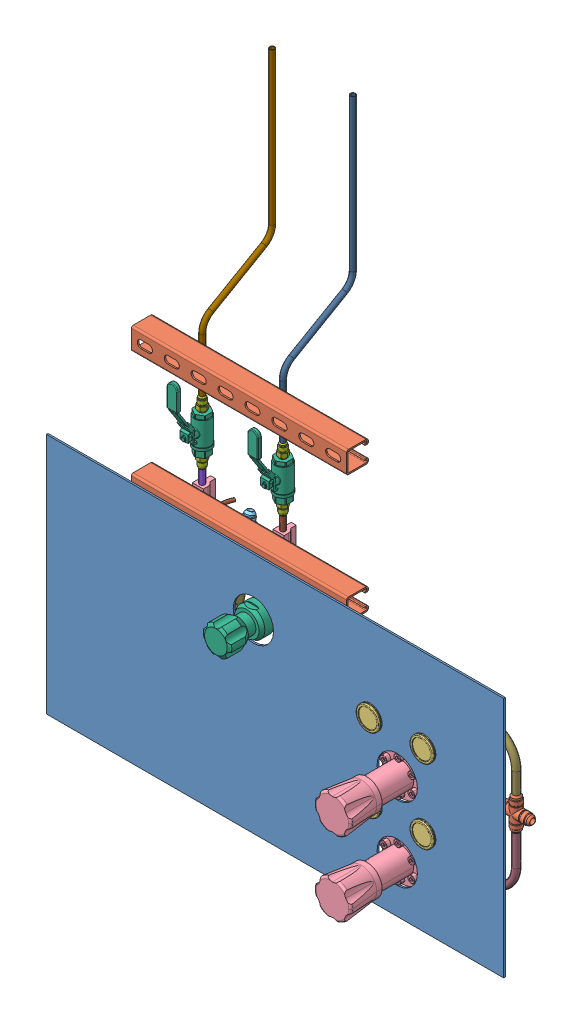
SolidWorks assembly N2_panel, configuration Default. Lengths in mm.
Overall size (886.81 1079.1 374.6).
81 component instances, 31 part files, 49 mates.
Components (placement in the parent):
- N2_panel-1: N2_panel [Default] at origin size (863.6 457.2 3.17)
- SS-2650-08-08-08-08-1: SS-2650-08-08-08-08 [5482K249] at (400.8501 0 -51.435) size (81.9 81.9 19.05)
- 9780T219_VIBRATION-RESISTANT PRESSURE GAUGE-3: 9780T219_VIBRATION-RESISTANT PRESSURE GAUGE [9780T219] at (179.9381 -67.2228 8.636) x (-1 0 0) z (0 0 1) size (44.45 61.91 48.07)
- 9780T219_VIBRATION-RESISTANT PRESSURE GAUGE-4: 9780T219_VIBRATION-RESISTANT PRESSURE GAUGE [9780T219] at (281.5381 -67.2228 8.636) x (-1 0 0) z (0 0 1) size (44.45 61.91 48.07)
- PRV-1 & PRV-2 Assembly-1: PRV-1 & PRV-2 Assembly [Default] at (230.7381 -139.7 -104.521) size (144.32 78.02 230.14)
  - PRV-1&2_RSHN4-02-6-VVK-Swagelok-1: PRV-1&2_RSHN4-02-6-VVK-Swagelok [Default] at origin size (72 78.02 230.14)
  - 50715K166_TYPE 316 SS 37 DEGREE FLARED TUBE FITTING-1: 50715K166_TYPE 316 SS 37 DEGREE FLARED TUBE FITTING [50715K802] at (39.556 0 53.086) x (1 0 0) z (0 0.0006 1) size (55.21 25.66 22.23)
  - 50715K166_TYPE 316 SS 37 DEGREE FLARED TUBE FITTING-2: 50715K166_TYPE 316 SS 37 DEGREE FLARED TUBE FITTING [50715K802] at (-39.556 0 53.086) x (-1 0 0) z (0 -0.0006 -1) size (55.21 25.66 22.23)
- PRV-3 Assembly-1: PRV-3 Assembly [Default] at (-40.8559 120.65 -138.049) x (-1 0 0) z (0 0 1) size (149.78 55.88 212.09)
  - KCY1JPA412A20000_PRT_29-1: KCY1JPA412A20000_PRT_29 [Default] at origin size (56.39 55.88 212.09)
  - 51205K317_EXTREME-PRESSURE 316 SS THREADED PIPE FITTING-1: 51205K317_EXTREME-PRESSURE 316 SS THREADED PIPE FITTING [51205K317] at (-34.807 0 86.614) x (-1 0 0) z (0 0.601506 -0.798868) size (42.93 32.74 28.57)
  - 50715K166_TYPE 316 SS 37 DEGREE FLARED TUBE FITTING-1: 50715K166_TYPE 316 SS 37 DEGREE FLARED TUBE FITTING [50715K802] at (-59.826 0 86.614) x (-1 0 0) z (0 -0.969103 0.246658) size (55.21 25.66 22.23)
  - 50715K163_TYPE 316 SS 37 DEGREE FLARED TUBE FITTING-1: 50715K163_TYPE 316 SS 37 DEGREE FLARED TUBE FITTING [50715K163] at (29.187 0 86.614) size (46.32 18.33 15.88)
- IPA_N2_manifold_1-1: IPA_N2_manifold_1 [Default] at (13.0485 19.3777 -0.8427) x (1 0 0) z (0 0.258819 0.965926) size (242.25 227.42 41.98)
  - 50715K166_TYPE 316 SS 37 DEGREE FLARED TUBE FITTING-1: 50715K166_TYPE 316 SS 37 DEGREE FLARED TUBE FITTING [50715K802] at (18.6216 -140.563 -90.0408) x (1 0 0) z (0 -0.539316 0.842104) size (55.21 25.66 22.23)
  - 5627K623_BRASS MANIFOLD WITH OUTLETS ON ONE SIDE-1: 5627K623_BRASS MANIFOLD WITH OUTLETS ON ONE SIDE [5627K623] at (-69.8974 -140.563 -90.0408) x (0 0 -1) z (1 0 0) size (38.1 38.1 158.75)
  - 4443K732_HIGH-PRESSURE 316 SS THREADED PIPE FITTING-1: 4443K732_HIGH-PRESSURE 316 SS THREADED PIPE FITTING [4443K732] at (-50.8474 -125.958 -90.0408) x (0 -1 0) z (0.415851 0 0.909433) size (19.05 20.24 17.88)
  - Pressure_sensor_standin-1: Pressure_sensor_standin [Default] at (-50.8474 -98.1907 -90.0408) x (0 -1 0) z (0.600596 0 -0.799553) size (123.69 32.03 28.45)
  - HPRV-500_PSV-1,2-1: HPRV-500_PSV-1,2 [Default] at (-12.7474 26.061 -90.0408) x (0.240643 0 0.970614) z (0 -1 0) size (31.75 35.92 128.52)
  - 5482K122_PRECISION AN 37 DEGREE FLARED TUBE FITTING-1: 5482K122_PRECISION AN 37 DEGREE FLARED TUBE FITTING [5482K122] at (-88.9474 -114.0708 -90.0408) x (0 1 0) z (0 0 1) size (45.71 22 19.05)
  - 48805K460_PRECISION EXTREME-PRESSURE 316SS PIPE FITTING-1: 48805K460_PRECISION EXTREME-PRESSURE 316SS PIPE FITTING [48805K46] at (-12.7474 -110.464 -90.0408) x (0 -1 0) z (-0.516882 0 0.856057) size (42.93 33 28.57)
  - 50715K166_TYPE 316 SS 37 DEGREE FLARED TUBE FITTING-2: 50715K166_TYPE 316 SS 37 DEGREE FLARED TUBE FITTING [50715K802] at (-158.4164 -140.563 -90.0408) x (-1 0 0) z (0 -0.862244 -0.506493) size (55.21 25.66 22.23)
  - 50715K165_TYPE 316 SS 37 DEGREE FLARED TUBE FITTING-1: 50715K165_TYPE 316 SS 37 DEGREE FLARED TUBE FITTING [50715K165] at (-127.0474 -112.242 -90.0408) x (0 1 0) z (0.237205 0 0.97146) size (48.86 23.83 20.64)
  - 50715K166_TYPE 316 SS 37 DEGREE FLARED TUBE FITTING-3: 50715K166_TYPE 316 SS 37 DEGREE FLARED TUBE FITTING [50715K802] at (-12.7474 35.205 -90.0408) x (0 1 0) z (0.645788 0 0.763516) size (55.21 25.66 22.23)
- 9780T219_VIBRATION-RESISTANT PRESSURE GAUGE-5: 9780T219_VIBRATION-RESISTANT PRESSURE GAUGE [9780T219] at (-152.4 21.6772 8.636) size (44.45 61.91 48.07) (suppressed, hidden)
- 9780T219_VIBRATION-RESISTANT PRESSURE GAUGE-6: 9780T219_VIBRATION-RESISTANT PRESSURE GAUGE [9780T219] at (-76.2 21.6772 8.636) size (44.45 61.91 48.07) (suppressed, hidden)
- PRV-1 & PRV-2 Assembly-2: PRV-1 & PRV-2 Assembly [Default] at (-127 -76.1799 -125.3) x (-1 0 0) z (0 0 1) size (144.32 78.02 230.14) (suppressed, hidden)
  - PRV-1&2_RSHN4-02-6-VVK-Swagelok-1: PRV-1&2_RSHN4-02-6-VVK-Swagelok [Default] at origin size (72 78.02 230.14)
  - 50715K166_TYPE 316 SS 37 DEGREE FLARED TUBE FITTING-1: 50715K166_TYPE 316 SS 37 DEGREE FLARED TUBE FITTING [50715K802] at (39.556 0 53.086) x (1 0 0) z (0 0.0006 1) size (55.21 25.66 22.23)
  - 50715K166_TYPE 316 SS 37 DEGREE FLARED TUBE FITTING-2: 50715K166_TYPE 316 SS 37 DEGREE FLARED TUBE FITTING [50715K802] at (-39.556 0 53.086) x (-1 0 0) z (0 -0.0006 -1) size (55.21 25.66 22.23)
- N2_pilot_manifold-1: N2_pilot_manifold [Default] at (15.875 -66.675 -10.16) size (236.06 32.55 141.21)
  - 5784T133_ASME-CODE NCKL-PLTD BRASS POP-SAFETY VALVE-1: 5784T133_ASME-CODE NCKL-PLTD BRASS POP-SAFETY VALVE [5784T133] at (-394.716 187.325 -41.275) x (0 0.086231 0.996275) z (0 -0.996275 0.086231) size (19.05 66.64 20.16)
  - 4839K732_TYPE 303 STAINLESS STEEL MANIFOLD-1: 4839K732_TYPE 303 STAINLESS STEEL MANIFOLD [4839K732] at (-331.7875 187.325 -41.275) x (0 -1 0) z (1 0 0) size (31.75 32.09 149.63)
  - 50715K164_TYPE 316 SS 37 DEGREE FLARED TUBE FITTING-1: 50715K164_TYPE 316 SS 37 DEGREE FLARED TUBE FITTING [50715K164] at (-253.111 187.325 -41.275) size (46.58 22 19.05)
  - 5361K320_TYPE 304 STAINLESS STEEL BARBED HOSE FITTING-1: 5361K320_TYPE 304 STAINLESS STEEL BARBED HOSE FITTING [5361K32] at (-387.35 187.325 -63.5) x (-0.53642 -0.843951 0) z (0 0 -1) size (14.29 16.5 47.66)
  - Pressure_sensor_standin-1: Pressure_sensor_standin [Default] at (-276.225 187.325 -71.374) x (0 0 1) z (-0.999827 -0.018586 0) size (123.69 32.03 28.45)
  - 5361K320_TYPE 304 STAINLESS STEEL BARBED HOSE FITTING-2: 5361K320_TYPE 304 STAINLESS STEEL BARBED HOSE FITTING [5361K32] at (-365.125 187.325 -63.5) x (-0.53642 -0.843951 0) z (0 0 -1) size (14.29 16.5 47.66)
  - 5361K320_TYPE 304 STAINLESS STEEL BARBED HOSE FITTING-3: 5361K320_TYPE 304 STAINLESS STEEL BARBED HOSE FITTING [5361K32] at (-342.9 187.325 -63.5) x (-0.53642 -0.843951 0) z (0 0 -1) size (14.29 16.5 47.66)
  - 5361K320_TYPE 304 STAINLESS STEEL BARBED HOSE FITTING-4: 5361K320_TYPE 304 STAINLESS STEEL BARBED HOSE FITTING [5361K32] at (-320.675 187.325 -63.5) x (-0.53642 -0.843951 0) z (0 0 -1) size (14.29 16.5 47.66)
  - 5361K320_TYPE 304 STAINLESS STEEL BARBED HOSE FITTING-5: 5361K320_TYPE 304 STAINLESS STEEL BARBED HOSE FITTING [5361K32] at (-298.45 187.325 -63.5) x (-0.53642 -0.843951 0) z (0 0 -1) size (14.29 16.5 47.66)
- 3310T530_STRUT CHANNEL_16-1: 3310T530_STRUT CHANNEL_16 [3310T53] at (114.6011 177.8 0) x (0 0 1) z (0 1 0) size (41.27 41.27 406.4)
- 008T012-1: 008T012 [Default] at (114.6011 120.65 -51.435) x (0 1 0) z (-1 0 0) size (23.88 34.04 44.45)
- 008T012-2: 008T012 [Default] at (114.6011 -139.7 -51.435) x (0 1 0) z (-1 0 0) size (23.88 34.04 44.45)
- 3310T530_STRUT CHANNEL_16-2: 3310T530_STRUT CHANNEL_16 [3310T53] at (93.9636 182.5625 -38.1) x (0 0 1) z (1 0 0) size (41.27 41.27 406.4)
- 006T010-3: 006T010 [Default] at (-228.2989 182.5625 -87.757) x (1 0 0) z (0 1 0) size (20.83 28.7 44.45)
- 006T010-2: 006T010 [Default] at (-75.8989 182.5625 -87.757) x (1 0 0) z (0 1 0) size (20.83 28.7 44.45)
- 3310T530_STRUT CHANNEL_16-3: 3310T530_STRUT CHANNEL_16 [3310T53] at (93.9636 423.8625 -38.1) x (0 0 1) z (1 0 0) size (41.27 41.27 406.4)
- 9780T219_VIBRATION-RESISTANT PRESSURE GAUGE-9: 9780T219_VIBRATION-RESISTANT PRESSURE GAUGE [9780T219] at (281.5381 72.4772 8.636) x (-1 0 0) z (0 0 1) size (44.45 61.91 48.07)
- 9780T219_VIBRATION-RESISTANT PRESSURE GAUGE-10: 9780T219_VIBRATION-RESISTANT PRESSURE GAUGE [9780T219] at (179.9381 72.4772 8.636) x (-1 0 0) z (0 0 1) size (44.45 61.91 48.07)
- 008T012-4: 008T012 [Default] at (114.6011 0 -51.435) x (0 1 0) z (-1 0 0) size (23.88 34.04 44.45)
- PRV-1 & PRV-2 Assembly-4: PRV-1 & PRV-2 Assembly [Default] at (230.7381 0 -104.521) size (144.32 78.02 230.14)
  - PRV-1&2_RSHN4-02-6-VVK-Swagelok-1: PRV-1&2_RSHN4-02-6-VVK-Swagelok [Default] at origin size (72 78.02 230.14)
  - 50715K166_TYPE 316 SS 37 DEGREE FLARED TUBE FITTING-1: 50715K166_TYPE 316 SS 37 DEGREE FLARED TUBE FITTING [50715K802] at (39.556 0 53.086) x (1 0 0) z (0 0.0006 1) size (55.21 25.66 22.23)
  - 50715K166_TYPE 316 SS 37 DEGREE FLARED TUBE FITTING-2: 50715K166_TYPE 316 SS 37 DEGREE FLARED TUBE FITTING [50715K802] at (-39.556 0 53.086) x (-1 0 0) z (0 -0.0006 -1) size (55.21 25.66 22.23)
- LOX_N2_manifold_1-1: LOX_N2_manifold_1 [Default] at (-139.3515 159.0777 -0.8427) x (1 0 0) z (0 0.258819 0.965926) size (242.25 227.42 41.98)
  - 50715K166_TYPE 316 SS 37 DEGREE FLARED TUBE FITTING-1: 50715K166_TYPE 316 SS 37 DEGREE FLARED TUBE FITTING [50715K802] at (18.6216 -140.563 -90.0408) x (1 0 0) z (0 -0.539316 0.842104) size (55.21 25.66 22.23)
  - 5627K623_BRASS MANIFOLD WITH OUTLETS ON ONE SIDE-1: 5627K623_BRASS MANIFOLD WITH OUTLETS ON ONE SIDE [5627K623] at (-69.8974 -140.563 -90.0408) x (0 0 -1) z (1 0 0) size (38.1 38.1 158.75)
  - 4443K732_HIGH-PRESSURE 316 SS THREADED PIPE FITTING-1: 4443K732_HIGH-PRESSURE 316 SS THREADED PIPE FITTING [4443K732] at (-50.8474 -125.958 -90.0408) x (0 -1 0) z (0.415851 0 0.909433) size (19.05 20.24 17.88)
  - Pressure_sensor_standin-1: Pressure_sensor_standin [Default] at (-50.8474 -98.1907 -90.0408) x (0 -1 0) z (0.600596 0 -0.799553) size (123.69 32.03 28.45)
  - HPRV-500_PSV-1,2-1: HPRV-500_PSV-1,2 [Default] at (-12.7474 26.061 -90.0408) x (0.240643 0 0.970614) z (0 -1 0) size (31.75 35.92 128.52)
  - 5482K122_PRECISION AN 37 DEGREE FLARED TUBE FITTING-1: 5482K122_PRECISION AN 37 DEGREE FLARED TUBE FITTING [5482K122] at (-88.9474 -114.0708 -90.0408) x (0 1 0) z (0 0 1) size (45.71 22 19.05)
  - 48805K460_PRECISION EXTREME-PRESSURE 316SS PIPE FITTING-1: 48805K460_PRECISION EXTREME-PRESSURE 316SS PIPE FITTING [48805K46] at (-12.7474 -110.464 -90.0408) x (0 -1 0) z (-0.516882 0 0.856057) size (42.93 33 28.57)
  - 50715K166_TYPE 316 SS 37 DEGREE FLARED TUBE FITTING-2: 50715K166_TYPE 316 SS 37 DEGREE FLARED TUBE FITTING [50715K802] at (-158.4164 -140.563 -90.0408) x (-1 0 0) z (0 -0.862244 -0.506493) size (55.21 25.66 22.23)
  - 4757T730_HIGH-PRESSURE BRASS THREADED PIPE FITTING-1: 4757T730_HIGH-PRESSURE BRASS THREADED PIPE FITTING [4757T73] at (-127.0474 -122.021 -90.0408) x (0 1 0) z (0.804983 0 0.593298) size (19.81 20.16 17.46)
  - 50715K166_TYPE 316 SS 37 DEGREE FLARED TUBE FITTING-3: 50715K166_TYPE 316 SS 37 DEGREE FLARED TUBE FITTING [50715K802] at (-12.7474 35.205 -90.0408) x (0 1 0) z (0.89562 0 -0.44482) size (55.21 25.66 22.23)
- HV-1,2-3: HV-1,2 [Default] at (-147.2516 261.0926 -192.2929) x (-0.983779 0 -0.179384) z (0.179384 0 -0.983779) size (44.38 176.24 77.79)
  - 47275K410_ULTRA-HIGH-PRESSURE 316SS BALL VALVE-1: 47275K410_ULTRA-HIGH-PRESSURE 316SS BALL VALVE [47275K41] at (-88.9474 28.7849 -90.0408) x (-0.983779 0 0.179384) z (0 -1 0) size (31.75 73.28 141.48)
  - 5482K123_PRECISION AN 37 DEGREE FLARED TUBE FITTING-1: 5482K123_PRECISION AN 37 DEGREE FLARED TUBE FITTING [5482K123] at (-88.9474 -13.4426 -90.0408) x (0 -1 0) z (0.141466 0 0.989943) size (44.92 18.33 15.88)
  - 5482K123_PRECISION AN 37 DEGREE FLARED TUBE FITTING-2: 5482K123_PRECISION AN 37 DEGREE FLARED TUBE FITTING [5482K123] at (-88.9474 71.0124 -90.0408) x (0 1 0) z (-0.141466 0 -0.989943) size (44.92 18.33 15.88)
- HV-1,2-4: HV-1,2 [Default] at (-299.6516 261.0926 -192.2929) x (-0.983779 0 -0.179384) z (0.179384 0 -0.983779) size (44.38 176.24 77.79)
  - 47275K410_ULTRA-HIGH-PRESSURE 316SS BALL VALVE-1: 47275K410_ULTRA-HIGH-PRESSURE 316SS BALL VALVE [47275K41] at (-88.9474 28.7849 -90.0408) x (-0.983779 0 0.179384) z (0 -1 0) size (31.75 73.28 141.48)
  - 5482K123_PRECISION AN 37 DEGREE FLARED TUBE FITTING-1: 5482K123_PRECISION AN 37 DEGREE FLARED TUBE FITTING [5482K123] at (-88.9474 -13.4426 -90.0408) x (0 -1 0) z (0.141466 0 0.989943) size (44.92 18.33 15.88)
  - 5482K123_PRECISION AN 37 DEGREE FLARED TUBE FITTING-2: 5482K123_PRECISION AN 37 DEGREE FLARED TUBE FITTING [5482K123] at (-88.9474 71.0124 -90.0408) x (0 1 0) z (-0.141466 0 -0.989943) size (44.92 18.33 15.88)
- Tube_2-N2_node-002-1: Tube_2-N2_node-002 [Default] at origin size (514.71 949.1 228.54)
  - Tube-375X035_1^Tube_2-N2_node-002-1: Tube-375X035_1^Tube_2-N2_node-002 [Tube .375in OD X .035in Wall] at (-228.2989 230.1875 -87.757) x (0.707107 0 0.707107) z (0 -1 0) size (27.01 27.01 188.58) (virtual)
  - Tube-375X035_2^Tube_2-N2_node-002-1: Tube-375X035_2^Tube_2-N2_node-002 [Tube .375in OD X .035in Wall] at (-228.2989 349.5675 -87.757) x (0.707107 0 0.707107) z (0 1 0) size (102.85 102.85 500.93) (virtual)
  - Tube-375X035_3^Tube_2-N2_node-002-1: Tube-375X035_3^Tube_2-N2_node-002 [Tube .375in OD X .035in Wall] at (-75.8989 349.5675 -87.757) x (0.707107 0 0.707107) z (0 1 0) size (102.85 102.85 500.93) (virtual)
  - Tube-375X035^Tube_2-N2_node-002-2: Tube-375X035^Tube_2-N2_node-002 [Tube .375in OD X .035in Wall] at (-75.8989 -96.8627 -62.9132) x (0.694747 0.186157 0.694747) z (0 0.965926 -0.258819) size (53.06 51.58 323.57) (virtual)
- Tube_3-N2_node-1: Tube_3-N2_node [Default] at origin size (374.6 273.05 374.6)
  - Tube-500X049^Tube_3-N2_node-1: Tube-500X049^Tube_3-N2_node [Tube .500in OD X .049in Wall] at (400.8501 30.9499 -51.435) x (0.707107 0 0.707107) z (0 1 0) size (264.89 264.89 96.05) (virtual)
  - Tube-500X049_1^Tube_3-N2_node-1: Tube-500X049_1^Tube_3-N2_node [Tube .500in OD X .049in Wall] at (400.8501 -30.9499 -51.435) x (0.707107 0 0.707107) z (0 -1 0) size (255.9 255.9 115.1) (virtual)
Mates (geometry in assembly coordinates):
- Coincident24: coincident anti-aligned: plane of Pressure_panel-1 through (0 0 3.175) normal (0 0 1); circle of 9780T219_VIBRATION-RESISTANT PRESSURE GAUGE-3
- Parallel12: parallel anti-aligned: plane of 9780T219_VIBRATION-RESISTANT PRESSURE GAUGE-4 through (273.0631 -36.2665 -18.7643) normal (-1 0 0)
- Parallel13: parallel aligned: plane of PRV-1 & PRV-2 Assembly-1/PRV-1&2_RSHN4-02-6-VVK-Swagelok-1 through (266.7381 -139.7 20.691) normal (1 0 0)
- Distance4: distance = 38.1 mm anti-aligned: plane of 9780T219_VIBRATION-RESISTANT PRESSURE GAUGE-3 through (183.0543 -72.6203 -29.718) normal (0 -1 0); plane of PRV-1 & PRV-2 Assembly-1/PRV-1&2_RSHN4-02-6-VVK-Swagelok-1 through (230.7381 -110.7203 -51.435) normal (0 1 0)
- Parallel18: parallel aligned: plane of SS-2650-08-08-08-08-1 through (400.8501 0 -51.435) normal (0 0 1)
- Distance9: distance = 50.8 mm anti-aligned: plane of 9780T219_VIBRATION-RESISTANT PRESSURE GAUGE-3 through (179.9381 -67.2228 8.636) normal (-1 0 0); plane of PRV-1 & PRV-2 Assembly-1/PRV-1&2_RSHN4-02-6-VVK-Swagelok-1 through (230.7381 -139.7 -104.521) normal (1 0 0)
- Coincident69: coincident anti-aligned: plane of Pressure_panel-1 through (0 0 0) normal (0 0 -1); plane of 3310T530_STRUT CHANNEL_16-1 through (131.7779 -228.6 0) normal (0 0 1)
- Coincident74: coincident aligned: plane of Pressure_panel-1 through (-431.8 -228.6 3.175) normal (0 -1 0); plane of 3310T530_STRUT CHANNEL_16-1 through (130.1904 -228.6 -36.2268) normal (0 -1 0)
- Coincident72: coincident anti-aligned: plane of 3310T530_STRUT CHANNEL_16-1 through (99.0119 -228.6 -41.275) normal (0 0 -1); plane of 008T012-1 through (92.3761 132.588 -41.275) normal (0 0 1)
- Coincident75: coincident aligned: plane of 008T012-1 through (136.8261 120.65 -51.435) normal (1 0 0); plane of 008T012-2 through (136.8261 -139.7 -51.435) normal (1 0 0)
- Coincident76: coincident aligned: plane of 008T012-1 through (92.3761 117.475 -75.311) normal (0 0 -1); plane of 008T012-2 through (92.3761 -142.875 -75.311) normal (0 0 -1)
- Distance21: distance = 1.5875 mm aligned: plane of 008T012-1 through (136.8261 120.65 -51.435) normal (1 0 0); plane of 3310T530_STRUT CHANNEL_16-1 through (135.2386 -228.6 -36.2268) normal (1 0 0)
- Coincident84: coincident aligned: plane of Pressure_panel-1 through (431.8 228.6 3.175) normal (1 0 0); plane of SS-2650-08-08-08-08-1 through (431.8 0 -51.435) normal (1 0 0)
- Concentric46: concentric anti-aligned: cone of PRV-1 & PRV-2 Assembly-1/PRV-1&2_RSHN4-02-6-VVK-Swagelok-1 through (259.2268 -139.7 -51.435) axis (-1 0 0); cylinder of 008T012-2 through (92.3761 -139.7 -51.435) axis (1 0 0) radius 6.35
- Distance23: distance = 107.95 mm aligned: plane of SS-2650-08-08-08-08-1 through (400.8501 0 -51.435) normal (1 0 0); plane of PRV-1 & PRV-2 Assembly-1/50715K802-1 through (292.9001 -139.7 -51.435) normal (1 0 0)
- Concentric47: concentric aligned: cylinder of IPA_N2_manifold_1-1/5627K623_BRASS MANIFOLD WITH OUTLETS ON ONE SIDE-1 through (31.6542 -139.7 -51.435) axis (1 0 0) radius 9.1281; cylinder of 008T012-2 through (92.3761 -139.7 -51.435) axis (1 0 0) radius 6.35
- Distance24: distance = 31.75 mm anti-aligned: plane of 008T012-2 through (136.8261 -139.7 -51.435) normal (1 0 0); plane of PRV-1 & PRV-2 Assembly-1/50715K802-2 through (168.5761 -139.7 -51.435) normal (-1 0 0)
- Concentric48: concentric aligned: cylinder of PRV-3 Assembly-1/50715K166_TYPE 316 SS 37 DEGREE FLARED TUBE FITTING-1 through (41.5761 120.65 -51.435) axis (1 0 0) radius 4.953; cylinder of 008T012-1 through (92.3761 120.65 -51.435) axis (1 0 0) radius 6.35
- Parallel37: parallel aligned: plane of N2_pilot_manifold-1 through (15.875 -66.675 -10.16) normal (0 1 0)
- Concentric49: concentric anti-aligned: cylinder of PRV-3 Assembly-1/50715K163_TYPE 316 SS 37 DEGREE FLARED TUBE FITTING-1 through (-51.8819 120.65 -51.435) axis (1 0 0) radius 7.1437; cylinder of N2_pilot_manifold-1/50715K164_TYPE 316 SS 37 DEGREE FLARED TUBE FITTING-1 through (-255.524 120.65 -51.435) axis (-1 0 0) radius 7.1437
- Distance27: distance = 38.1 mm anti-aligned: plane of Pressure_panel-1 through (0 0 0) normal (0 0 -1); plane of 3310T530_STRUT CHANNEL_16-2 through (-312.4364 165.3858 -38.1) normal (0 0 1)
- Distance35: distance = 25.4 mm aligned: plane of Pressure_panel-1 through (-431.8 228.6 3.175) normal (0 1 0); plane of 3310T530_STRUT CHANNEL_16-2 through (-312.4364 203.2 -74.3268) normal (0 1 0)
- Coincident93: coincident anti-aligned: plane of 3310T530_STRUT CHANNEL_16-1 through (93.9636 -228.6 -36.2268) normal (-1 0 0); plane of 3310T530_STRUT CHANNEL_16-2 through (93.9636 166.9732 -74.3268) normal (1 0 0)
- Parallel38: parallel anti-aligned: plane of PRV-3 Assembly-1 through (-40.8559 120.65 -138.049) normal (0 -1 0)
- Concentric50: concentric anti-aligned: cylinder of PRV-1 & PRV-2 Assembly-4/50715K166_TYPE 316 SS 37 DEGREE FLARED TUBE FITTING-2 through (213.7881 0 -51.435) axis (1 0 0) radius 9.525; cylinder of LOX_N2_manifold_1-1/50715K166_TYPE 316 SS 37 DEGREE FLARED TUBE FITTING-1 through (-143.3359 0 -51.435) axis (-1 0 0) radius 9.525
- Parallel39: parallel aligned: plane of IPA_N2_manifold_1-1/5627K623_BRASS MANIFOLD WITH OUTLETS ON ONE SIDE-1 through (22.5261 -163.0314 -64.9054) normal (0 -0.258819 -0.965926); plane of LOX_N2_manifold_1-1/5627K623_BRASS MANIFOLD WITH OUTLETS ON ONE SIDE-1 through (-129.8739 -23.3314 -64.9054) normal (0 -0.258819 -0.965926)
- Distance28: distance = 88.9 mm: plane of PRV-1 & PRV-2 Assembly-1 through (230.7381 -139.7 -104.521) normal (0 1 0); line of Pressure_panel-1 through (-431.8 -228.6 3.175) axis (1 0 0)
- Angle1: planar angle = 0.261799 rad aligned: plane of IPA_N2_manifold_1-1/5627K623_BRASS MANIFOLD WITH OUTLETS ON ONE SIDE-1 through (22.5261 -163.0314 -64.9054) normal (0 -0.258819 -0.965926); plane of Pressure_panel-1 through (0 0 0) normal (0 0 -1)
- Coincident96: coincident anti-aligned: plane of 3310T530_STRUT CHANNEL_16-2 through (-312.4364 198.1517 -79.375) normal (0 0 -1); plane of 006T010-3 through (-217.8849 204.7875 -79.375) normal (0 0 1)
- Distance29: distance = 1.5875 mm aligned: plane of 3310T530_STRUT CHANNEL_16-2 through (-312.4364 203.2 -74.3268) normal (0 1 0); plane of 006T010-3 through (-228.2989 204.7875 -87.757) normal (0 1 0)
- Coincident98: coincident anti-aligned: plane of LOX_N2_manifold_1-1/5482K122_PRECISION AN 37 DEGREE FLARED TUBE FITTING-1 through (-228.2989 25.5895 -58.2917) normal (-1 0 0); plane of 006T010-3 through (-228.2989 182.5625 -87.757) normal (1 0 0)
- Distance30: distance = 38.1 mm anti-aligned: plane of IPA_N2_manifold_1-1/50715K802-1 through (54.2761 -139.7 -51.435) normal (1 0 0); plane of 008T012-2 through (92.3761 -139.7 -51.435) normal (-1 0 0)
- Coincident101: coincident aligned: plane of 006T010-3 through (-232.9979 204.7875 -108.077) normal (0 0 -1); plane of 006T010-2 through (-80.5979 204.7875 -108.077) normal (0 0 -1)
- Coincident102: coincident aligned: plane of 006T010-3 through (-228.2989 204.7875 -87.757) normal (0 1 0); plane of 006T010-2 through (-75.8989 204.7875 -87.757) normal (0 1 0)
- Coincident103: coincident anti-aligned: plane of IPA_N2_manifold_1-1/5482K122_PRECISION AN 37 DEGREE FLARED TUBE FITTING-1 through (-75.8989 -114.1105 -58.2917) normal (-1 0 0); plane of 006T010-2 through (-75.8989 182.5625 -87.757) normal (1 0 0)
- Concentric51: concentric anti-aligned: cylinder of 006T010-2 through (-75.8989 204.7875 -87.757) axis (0 -1 0) radius 4.699; cylinder of HV-1,2-3/5482K123_PRECISION AN 37 DEGREE FLARED TUBE FITTING-1 through (-75.8989 265.1125 -87.757) axis (0 1 0) radius 7.1437
- Concentric52: concentric anti-aligned: cylinder of 006T010-3 through (-228.2989 204.7875 -87.757) axis (0 -1 0) radius 4.699; cylinder of HV-1,2-4/5482K123_PRECISION AN 37 DEGREE FLARED TUBE FITTING-1 through (-228.2989 265.1125 -87.757) axis (0 1 0) radius 7.1437
- Coincident106: coincident aligned: plane of HV-1,2-3/47275K410_ULTRA-HIGH-PRESSURE 316SS BALL VALVE-1 through (-75.8989 324.8025 -87.757) normal (0 1 0); plane of HV-1,2-4/47275K410_ULTRA-HIGH-PRESSURE 316SS BALL VALVE-1 through (-228.2989 324.8025 -87.757) normal (0 1 0)
- Distance31: distance = 152.4 mm aligned: plane of 006T010-3 through (-238.7129 204.7875 -79.375) normal (-1 0 0); plane of 006T010-2 through (-86.3129 204.7875 -79.375) normal (-1 0 0)
- Distance32: distance = 260.35 mm aligned: plane of 008T012-1 through (92.3761 132.588 -51.435) normal (0 1 0); plane of 008T012-2 through (92.3761 -127.762 -51.435) normal (0 1 0)
- Distance34: distance = 12.7 mm aligned: plane of PRV-3 Assembly-1/50715K802-1 through (41.5761 120.65 -51.435) normal (1 0 0); plane of IPA_N2_manifold_1-1/50715K802-1 through (54.2761 -139.7 -51.435) normal (1 0 0)
- Distance33: distance = 25.4 mm anti-aligned: plane of 006T010-3 through (-228.2989 204.7875 -87.757) normal (0 1 0); plane of HV-1,2-4/5482K123_PRECISION AN 37 DEGREE FLARED TUBE FITTING-1 through (-228.2989 230.1875 -87.757) normal (0 -1 0)
- Parallel43: parallel aligned: plane of HV-1,2-3/47275K410_ULTRA-HIGH-PRESSURE 316SS BALL VALVE-1 through (-75.8989 289.8775 -87.757) normal (0 0 1)
- Parallel44: parallel aligned: plane of HV-1,2-4/47275K410_ULTRA-HIGH-PRESSURE 316SS BALL VALVE-1 through (-228.2989 289.8775 -87.757) normal (0 0 1)
- Concentric53: concentric aligned: cylinder of SS-2650-08-08-08-08-1 through (400.8501 0 -51.435) axis (-1 0 0) radius 9.525; cylinder of PRV-1 & PRV-2 Assembly-4/50715K166_TYPE 316 SS 37 DEGREE FLARED TUBE FITTING-1 through (247.6881 0 -51.435) axis (-1 0 0) radius 9.525
- Coincident112: coincident aligned: plane of 3310T530_STRUT CHANNEL_16-2 through (93.9636 166.9732 -74.3268) normal (1 0 0); plane of 3310T530_STRUT CHANNEL_16-3 through (93.9636 408.2732 -74.3268) normal (1 0 0)
- Coincident113: coincident aligned: plane of 3310T530_STRUT CHANNEL_16-2 through (-312.4364 165.3858 -38.1) normal (0 0 1); plane of 3310T530_STRUT CHANNEL_16-3 through (-312.4364 406.6857 -38.1) normal (0 0 1)
- Distance36: distance = 241.3 mm aligned: plane of 3310T530_STRUT CHANNEL_16-2 through (-312.4364 203.2 -74.3268) normal (0 1 0); plane of 3310T530_STRUT CHANNEL_16-3 through (-312.4364 444.5 -74.3268) normal (0 1 0)
- Distance37: distance = 41.275 mm aligned: plane of N2_pilot_manifold-1/4839K732_TYPE 303 STAINLESS STEEL MANIFOLD-1 through (-390.525 136.525 -67.31) normal (-1 0 0); plane of Pressure_panel-1 through (-431.8 228.6 3.175) normal (-1 0 0)
